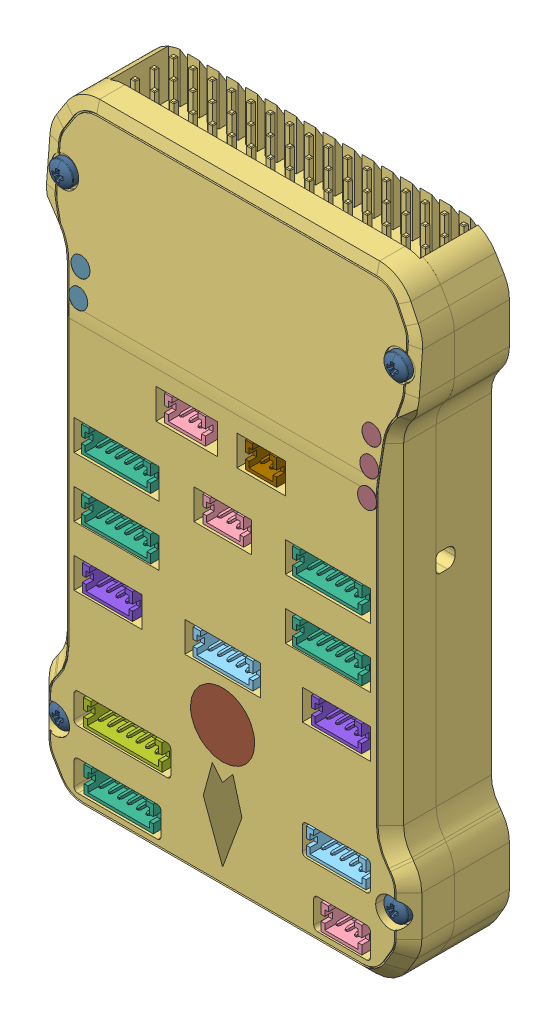
SolidWorks assembly PIXHAWK, configuration Default. Lengths in mm.
Overall size (62.89 81.3 15.33).
27 component instances, 14 part files, 0 mates.
Components (placement in the parent):
- Pixhawk.STEP-1: Pixhawk.STEP [Default] at origin size (62.89 81.3 15.33)
  - micro USB.STEP-1: micro USB.STEP [Default] at (-38.5288 4.0262 13.8589) x (0 1 0) z (-1 0 0) size (21.92 8.86 21.44)
    - micro usb02.STEP-1: micro usb02.STEP [Default] at (-14.4796 6.4719 -20.7085) size (6.9 2.16 4.2)
    - micro usb.STEP-1: micro usb.STEP [Default] at (-14.4796 6.4719 -16.0085) size (7.98 2.93 5.44)
  - Pixhawk APM.STEP-1: Pixhawk APM.STEP [Default] at (-25.3722 -39.1501 0) size (49.31 81.3 15.02)
  - DF13-3P-1.25DSA.STEP-1: DF13-3P-1.25DSA.STEP [Default] at (0.001 -60.127 12.2305) x (0 -1 0) z (-1 0 0) size (3.41 6.61 5.41)
  - DF13-5P-1.25DSA.STEP-1: DF13-5P-1.25DSA.STEP [Default] at (0.5502 -52.3839 12.2305) x (0 -1 0) z (-1 0 0) size (3.41 6.61 7.91)
  - DF13-6P-1.25DSA.STEP-1: DF13-6P-1.25DSA.STEP [Default] at (-27.5951 -60.0382 12.2305) x (0 -1 0) z (-1 0 0) size (3.41 6.61 9.16)
  - DF13-7P-1.25DSA.STEP-1: DF13-7P-1.25DSA.STEP [Default] at (-26.4213 -52.4032 12.2305) x (0 -1 0) z (-1 0 0) size (3.41 6.61 10.41)
  - DF13-4P-1.25DSA.STEP-1: DF13-4P-1.25DSA.STEP [Default] at (-0.0265 -37.0823 12.2305) x (0 -1 0) z (-1 0 0) size (3.41 6.61 6.66)
  - DF13-4P-1.25DSA.STEP-2: DF13-4P-1.25DSA.STEP [Default] at (-30.3382 -37.0823 12.2305) x (0 -1 0) z (-1 0 0) size (3.41 6.61 6.66)
  - DF13-5P-1.25DSA.STEP-2: DF13-5P-1.25DSA.STEP [Default] at (-14.4216 -37.0823 12.2305) x (0 -1 0) z (-1 0 0) size (3.41 6.61 7.91)
  - DF13-6P-1.25DSA.STEP-2: DF13-6P-1.25DSA.STEP [Default] at (-0.012 -29.2904 12.2305) x (0 -1 0) z (-1 0 0) size (3.41 6.61 9.16)
  - DF13-6P-1.25DSA.STEP-3: DF13-6P-1.25DSA.STEP [Default] at (-0.012 -21.2194 12.2305) x (0 -1 0) z (-1 0 0) size (3.41 6.61 9.16)
  - DF13-6P-1.25DSA.STEP-4: DF13-6P-1.25DSA.STEP [Default] at (-27.948 -29.2904 12.2305) x (0 -1 0) z (-1 0 0) size (3.41 6.61 9.16)
  - DF13-6P-1.25DSA.STEP-5: DF13-6P-1.25DSA.STEP [Default] at (-27.948 -21.2194 12.2305) x (0 -1 0) z (-1 0 0) size (3.41 6.61 9.16)
  - DF13-3P-1.25DSA.STEP-2: DF13-3P-1.25DSA.STEP [Default] at (-15.6441 -21.2194 12.2305) x (0 -1 0) z (-1 0 0) size (3.41 6.61 5.41)
  - DF13-2P-1.25DSA.STEP-1: DF13-2P-1.25DSA.STEP [Default] at (-11.2684 -12.1811 12.2305) x (0 -1 0) z (-1 0 0) size (3.41 6.61 4.16)
  - DF13-3P-1.25DSA.STEP-3: DF13-3P-1.25DSA.STEP [Default] at (-20.7011 -12.1811 12.2305) x (0 -1 0) z (-1 0 0) size (3.41 6.61 5.41)
  - pan head cross recess screw_iso_ISO 7045 - M1.6 x 3 - Z --- 3N.STEP-1: pan head cross recess screw_iso_ISO 7045 - M1.6 x 3 - Z --- 3N.STEP [Default] at (21.4278 32.5499 14.8) x (0 0 -1) z (1 0 0) size (4.27 3.2 3.2)
  - pan head cross recess screw_iso_ISO 7045 - M1.6 x 3 - Z --- 3N.STEP-2: pan head cross recess screw_iso_ISO 7045 - M1.6 x 3 - Z --- 3N.STEP [Default] at (-22.8722 32.5499 14.8) x (0 0 -1) z (1 0 0) size (4.27 3.2 3.2)
  - pan head cross recess screw_iso_ISO 7045 - M1.6 x 3 - Z --- 3N.STEP-3: pan head cross recess screw_iso_ISO 7045 - M1.6 x 3 - Z --- 3N.STEP [Default] at (21.4278 -29.5501 14.8) x (0 0 -1) z (1 0 0) size (4.27 3.2 3.2)
  - pan head cross recess screw_iso_ISO 7045 - M1.6 x 3 - Z --- 3N.STEP-4: pan head cross recess screw_iso_ISO 7045 - M1.6 x 3 - Z --- 3N.STEP [Default] at (-22.8722 -29.5501 14.8) x (0 0 -1) z (1 0 0) size (4.27 3.2 3.2)
  - Pi_ce10^Pixhawk.STEP-1: Pi_ce10^Pixhawk.STEP [Default] at (-25.3722 -39.1501 14.5) size (8.5 8.5 0.5)
  - Pi_ce11^Pixhawk.STEP-1: Pi_ce11^Pixhawk.STEP [Default] at (-25.3722 -39.1501 14.5) size (5.12 11.31 0.5)
  - Pi_ce12^Pixhawk.STEP-1: Pi_ce12^Pixhawk.STEP [Default] at (-25.3722 -37.5551 19.1403) x (1 0 0) z (0 0.083045 0.996546) size (2.5 9.53 0.5)
  - Pi_ce13^Pixhawk.STEP-1: Pi_ce13^Pixhawk.STEP [Default] at (-25.3722 -37.5551 19.1403) x (1 0 0) z (0 0.083045 0.996546) size (2.5 6.02 0.5)
